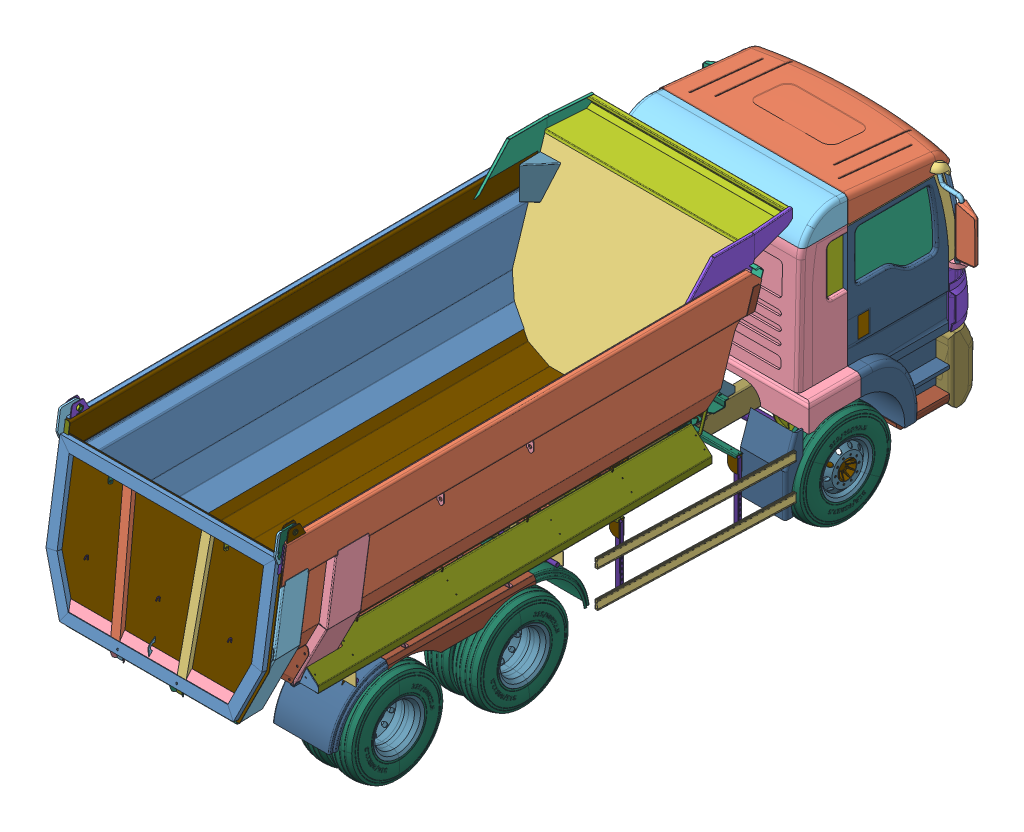
SolidWorks assembly MAN5, configuration Default. Lengths in mm. (continued)
Components (placement in the parent): (continued)
- MAN5.IGS-1: MAN5.IGS [Default] at origin size (3197.79 4674.46 9356.54) (continued)
  - M5 - erp33360_kapak üst sallama 20mm.IGS-1: M5 - erp33360_kapak üst sallama 20mm.IGS [Default] at (1250.8381 2990.2578 7990.13) x (0 0.005539 -0.999985) z (1 0 0) size (234.68 267.08 20.01)
  - M5 - erp33360_ÖZBEK SALLAMA MÝL.IGS-1: M5 - erp33360_ÖZBEK SALLAMA MÝL.IGS [Default] at (1196.3523 3240.9663 7706.3093) x (-1 0 0) z (0 0.043618 -0.999048) size (108.47 50 50)
  - M5 - erp33360_BURÇ1.IGS-1: M5 - erp33360_BURÇ1.IGS [Default] at (1169.8381 3240.9663 7706.3093) x (0 0.043618 -0.999048) z (1 0 0) size (57.01 57.11 25.54)
  - M5 - erp33360_sallama ayak.IGS-1: M5 - erp33360_sallama ayak.IGS [Default] at (1268.8381 3095.3253 7892.1663) x (0 0.005539 -0.999985) z (1 0 0) size (210.07 125.51 8.51)
  - M5 - erp33360_sallama ayak.IGS-2: M5 - erp33360_sallama ayak.IGS [Default] at (1205.8381 3095.3253 7892.1663) x (0 0.005539 -0.999985) z (1 0 0) size (210.07 125.51 8.51)
  - M5 - erp33360_BURÇ2.IGS-1: M5 - erp33360_BURÇ2.IGS [Default] at (1215.8381 3240.9663 7706.3093) x (0 0.879079 0.476677) z (1 0 0) size (57 57 45.54)
  - M5 - erp33360_BURÇ PÝMÝ.IGS-1: M5 - erp33360_BURÇ PÝMÝ.IGS [Default] at (1182.8381 3218.1971 7705.3152) x (0 -0.999048 -0.043618) z (0 0.043618 -0.999048) size (88.01 16.63 20.01)
  - M5 - erp33360_PÝM.IGS-1: M5 - erp33360_PÝM.IGS [Default] at (1182.2163 3195.6645 7744.3361) x (0 -0.043618 0.999048) z (0 -0.999048 -0.043618) size (56.72 5.64 2.41)
  - M5 - erp33360_Sallama ara parça.IGS-1: M5 - erp33360_Sallama ara parça.IGS [Default] at (1268.8381 3241.0739 7621.6777) x (-1 0 0) z (0 0.474355 -0.880334) size (55.01 80.01 5.01)
  - M5 - erp33360_kapak_Ust_Sallama_20mm_yený.IGS-1: M5 - erp33360_kapak_Ust_Sallama_20mm_yený.IGS [Default] at (1250.8381 3240.9663 7706.3093) x (0 0.006563 -0.999978) z (1 0 0) size (258.68 309.94 20.01)
  - M5 - erp33360_kapak_Ust_Sallama_20mm_yený.IGS-2: M5 - erp33360_kapak_Ust_Sallama_20mm_yený.IGS [Default] at (-1179.1619 3240.9663 7706.3093) x (0 0.006563 -0.999978) z (1 0 0) size (258.68 309.94 20.01)
  - M5 - erpAynalama33360_ÖZBEK SALLAMA MÝL.IGS-1: M5 - erpAynalama33360_ÖZBEK SALLAMA MÝL.IGS [Default] at (-1144.6762 3240.9663 7706.3093) x (1 0 0) z (0 -0.043618 0.999048) size (108.47 50 50)
  - M5 - erpAynalama33360_BURÇ1.IGS-1: M5 - erpAynalama33360_BURÇ1.IGS [Default] at (-1118.1619 3240.9663 7706.3093) x (0 0.043618 -0.999048) z (1 0 0) size (57.01 57.11 25.01)
  - M5 - erpAynalama33360_sallama ayak.IGS-1: M5 - erpAynalama33360_sallama ayak.IGS [Default] at (-1217.1619 3095.3253 7892.1663) x (0 0.005539 -0.999985) z (1 0 0) size (210.07 125.01 8.01)
  - M5 - erpAynalama33360_sallama ayak.IGS-2: M5 - erpAynalama33360_sallama ayak.IGS [Default] at (-1154.1619 3095.3253 7892.1663) x (0 0.005539 -0.999985) z (1 0 0) size (210.07 125.01 8.01)
  - M5 - erpAynalama33360_BURÇ2.IGS-1: M5 - erpAynalama33360_BURÇ2.IGS [Default] at (-1164.1619 3240.9663 7706.3093) x (0 0.879079 0.476677) z (1 0 0) size (57 57 45.54)
  - M5 - erpAynalama33360_BURÇ PÝMÝ.IGS-1: M5 - erpAynalama33360_BURÇ PÝMÝ.IGS [Default] at (-1131.1619 3218.1971 7705.3152) x (0 -0.999048 -0.043618) z (0 -0.043618 0.999048) size (88.01 16.63 20.01)
  - M5 - erpAynalama33360_PÝM.IGS-1: M5 - erpAynalama33360_PÝM.IGS [Default] at (-1130.5402 3195.6645 7744.3361) x (0 -0.043618 0.999048) z (0 0.999048 0.043618) size (56.72 5.64 2.41)
  - M5 - erpAynalama33360_Sallama ara parça.IGS-1: M5 - erpAynalama33360_Sallama ara parça.IGS [Default] at (-1217.1619 3241.0739 7621.6777) x (1 0 0) z (0 -0.474355 0.880334) size (55.01 80.01 5.01)
  - M5 - erp33360_kapak kilitleme dili.IGS-1: M5 - erp33360_kapak kilitleme dili.IGS [Default] at (-520.9865 1303.6235 8070.908) x (1 0 0) z (0 -0.050827 0.998707) size (166.16 71.61 59.75)
  - M5 - erp33360_dil iç takviye.IGS-1: M5 - erp33360_dil iç takviye.IGS [Default] at (-468.4024 1337.6943 8080.6523) x (1 0 0) z (0 -0.050827 0.998707) size (76.08 56.18 8.01)
  - M5 - erpAynalama33360_kapak kilitleme dili.IGS-1: M5 - erpAynalama33360_kapak kilitleme dili.IGS [Default] at (572.6626 1303.6235 8070.908) x (-1 0 0) z (0 0.050827 -0.998707) size (166.16 71.61 64.28)
  - M5 - erpAynalama33360_dil iç takviye.IGS-1: M5 - erpAynalama33360_dil iç takviye.IGS [Default] at (520.0785 1337.6943 8080.6523) x (-1 0 0) z (0 0.050827 -0.998707) size (76.08 56.18 8.01)
  - M5 - erp33360_kanca.IGS-1: M5 - erp33360_kanca.IGS [Default] at (-1007.12 1894.6124 3041.2431) x (-0.707107 -0.707096 -0.003916) z (0 0.005539 -0.999985) size (48.6 48.28 20.01)
  - M5 - erp33360_kanca.IGS-2: M5 - erp33360_kanca.IGS [Default] at (-1007.12 1889.3508 3991.2285) x (-0.707107 -0.707096 -0.003916) z (0 0.005539 -0.999985) size (48.6 48.28 20.01)
  - M5 - erp33360_kanca.IGS-3: M5 - erp33360_kanca.IGS [Default] at (-1007.12 1884.0892 4941.214) x (-0.707107 -0.707096 -0.003916) z (0 0.005539 -0.999985) size (48.6 48.28 20.01)
  - M5 - erp33360_kanca.IGS-4: M5 - erp33360_kanca.IGS [Default] at (-1007.12 1878.8276 5891.1994) x (-0.707107 -0.707096 -0.003916) z (0 0.005539 -0.999985) size (48.6 48.28 20.01)
  - M5 - erp33360_kanca.IGS-5: M5 - erp33360_kanca.IGS [Default] at (-1007.12 1873.566 6841.1848) x (-0.707107 -0.707096 -0.003916) z (0 0.005539 -0.999985) size (48.6 48.28 20.01)
  - M5 - erp33360_kanca.IGS-6: M5 - erp33360_kanca.IGS [Default] at (-1007.12 1869.1352 7641.1725) x (-0.707107 -0.707096 -0.003916) z (0 0.005539 -0.999985) size (48.6 48.28 20.01)
  - M5 - erp33360_kanca.IGS-7: M5 - erp33360_kanca.IGS [Default] at (-995.483 2108.1822 2887.3964) x (0 -0.303745 -0.952753) z (0.927289 0.35666 -0.113706) size (48.6 48.28 20.01)
  - M5 - erp33360_kanca.IGS-8: M5 - erp33360_kanca.IGS [Default] at (-962.1619 3328.5865 2328.3233) x (0 -0.999985 -0.005539) z (1 0 0) size (48.6 48.28 20.01)
  - M5 - erp33360_kanca.IGS-9: M5 - erp33360_kanca.IGS [Default] at (-312.1619 3328.5865 2328.3233) x (0 -0.999985 -0.005539) z (1 0 0) size (48.6 48.28 20.01)
  - M5 - erp33360_kanca.IGS-10: M5 - erp33360_kanca.IGS [Default] at (-774.1619 2086.9433 7981.607) x (0 0.150962 0.98854) z (-1 0 0) size (48.6 48.28 20.01)
  - M5 - erp33360_kanca.IGS-11: M5 - erp33360_kanca.IGS [Default] at (25.8381 2086.9433 7981.607) x (0 0.150962 0.98854) z (-1 0 0) size (48.6 48.28 20.01)
  - M5 - erp33360_kanca.IGS-12: M5 - erp33360_kanca.IGS [Default] at (825.8381 2086.9433 7981.607) x (0 0.150962 0.98854) z (-1 0 0) size (48.6 48.28 20.01)
  - M5 - erpAynalama33360_kanca.IGS-1: M5 - erpAynalama33360_kanca.IGS [Default] at (1047.1591 2108.1822 2887.3964) x (0 -0.303745 -0.952753) z (0.927289 -0.35666 0.113706) size (48.6 48.28 20.01)
  - M5 - erpAynalama33360_kanca.IGS-2: M5 - erpAynalama33360_kanca.IGS [Default] at (1058.7961 1894.6124 3041.2431) x (0.707107 -0.707096 -0.003916) z (0 -0.005539 0.999985) size (48.6 48.28 20.01)
  - M5 - erpAynalama33360_kanca.IGS-3: M5 - erpAynalama33360_kanca.IGS [Default] at (1058.7961 1889.3508 3991.2285) x (0.707107 -0.707096 -0.003916) z (0 -0.005539 0.999985) size (48.6 48.28 20.01)
  - M5 - erpAynalama33360_kanca.IGS-4: M5 - erpAynalama33360_kanca.IGS [Default] at (1058.7961 1884.0892 4941.214) x (0.707107 -0.707096 -0.003916) z (0 -0.005539 0.999985) size (48.6 48.28 20.01)
  - M5 - erpAynalama33360_kanca.IGS-5: M5 - erpAynalama33360_kanca.IGS [Default] at (1058.7961 1878.8276 5891.1994) x (0.707107 -0.707096 -0.003916) z (0 -0.005539 0.999985) size (48.6 48.28 20.01)
  - M5 - erpAynalama33360_kanca.IGS-6: M5 - erpAynalama33360_kanca.IGS [Default] at (1058.7961 1873.566 6841.1848) x (0.707107 -0.707096 -0.003916) z (0 -0.005539 0.999985) size (48.6 48.28 20.01)
  - M5 - erpAynalama33360_kanca.IGS-7: M5 - erpAynalama33360_kanca.IGS [Default] at (1058.7961 1869.1352 7641.1725) x (0.707107 -0.707096 -0.003916) z (0 -0.005539 0.999985) size (48.6 48.28 20.01)
  - M5 - erpAynalama33360_kanca.IGS-8: M5 - erpAynalama33360_kanca.IGS [Default] at (1013.8381 3328.5865 2328.3233) x (0 -0.999985 -0.005539) z (1 0 0) size (48.6 48.28 20.01)
  - M5 - erpAynalama33360_kanca.IGS-9: M5 - erpAynalama33360_kanca.IGS [Default] at (363.8381 3328.5865 2328.3233) x (0 -0.999985 -0.005539) z (1 0 0) size (48.6 48.28 20.01)
  - M5 - erp3360_kulak iç takviye.IGS-1: M5 - erp3360_kulak iç takviye.IGS [Default] at (-968.4538 1432.4795 7379.0946) x (1 0 0) z (0 -0.005539 0.999985) size (545.81 169.76 8.01)
  - M5 - erp3360_kulak iç takviye.IGS-2: M5 - erp3360_kulak iç takviye.IGS [Default] at (-968.4538 1433.6426 7169.0978) x (1 0 0) z (0 -0.005539 0.999985) size (545.81 169.76 8.01)
  - M5 - erpAynalama3360_kulak iç takviye.IGS-1: M5 - erpAynalama3360_kulak iç takviye.IGS [Default] at (1020.1299 1432.4795 7379.0946) x (-1 0 0) z (0 0.005539 -0.999985) size (545.81 169.76 8.01)
  - M5 - erpAynalama3360_kulak iç takviye.IGS-2: M5 - erpAynalama3360_kulak iç takviye.IGS [Default] at (1020.1299 1433.6426 7169.0978) x (-1 0 0) z (0 0.005539 -0.999985) size (545.81 169.76 8.01)
  - M5 - erp33360_Kulak iç L takviye.IGS-1: M5 - erp33360_Kulak iç L takviye.IGS [Default] at (685.8381 1536.3346 7100.1114) x (0 0.168191 0.985754) z (-1 0 0) size (40.01 60.01 250.01)
  - M5 - erpAynalama33360_Kulak iç L takviye.IGS-1: M5 - erpAynalama33360_Kulak iç L takviye.IGS [Default] at (685.8381 1534.4342 7443.2144) x (0 0.1791 -0.983831) z (1 0 0) size (40.01 60.01 250.01)
  - M5 - erpAynalama33360_Kulak iç L takviye.IGS-2: M5 - erpAynalama33360_Kulak iç L takviye.IGS [Default] at (-634.162 1536.3346 7100.1114) x (0 0.168191 0.985754) z (-1 0 0) size (40.01 60.01 250.01)
  - M5 - erpAynalamaAynalama33360_Kulak iç L takviye.IGS-1: M5 - erpAynalamaAynalama33360_Kulak iç L takviye.IGS [Default] at (-634.162 1534.4342 7443.2144) x (0 0.1791 -0.983831) z (1 0 0) size (40.01 60.01 250.01)
  - M5 - erp33360_takviye 3.IGS-1: M5 - erp33360_takviye 3.IGS [Default] at (496.575 1458.2519 7075.2326) x (-1 0 0) z (0 0.005539 -0.999985) size (707.09 63.73 70.86)
  - M5 - erpAynalama33360_takviye 3.IGS-1: M5 - erpAynalama33360_takviye 3.IGS [Default] at (496.575 1456.0808 7467.2266) x (-1 0 0) z (0 0.005539 -0.999985) size (707.09 63.73 70.86)
  - M5 - erp33360_takviye 2.IGS-1: M5 - erp33360_takviye 2.IGS [Default] at (-1807.7153 1265.8802 7061.7989) x (0.99991 -0.000074 0.013388) z (-0.013388 -0.000196 0.99991) size (761.79 408.47 64.91)
  - M5 - erp33360_takviye 2.IGS-2: M5 - erp33360_takviye 2.IGS [Default] at (-1807.7153 1263.6925 7456.7928) x (0.99991 -0.000074 0.013388) z (-0.013388 -0.000196 0.99991) size (761.79 408.47 64.91)
  - M5 - erp33360_takviye 1.IGS-1: M5 - erp33360_takviye 1.IGS [Default] at (-1188.2366 1554.8437 7093.9387) x (1 0 0) z (0 0.194032 0.980995) size (498.01 334.11 6.01)
  - M5 - erp33360_takviye 1.IGS-2: M5 - erp33360_takviye 1.IGS [Default] at (-1189.0116 1551.4786 7467.5378) x (1 0 0) z (0 0.177892 0.98405) size (498.01 334.11 6.01)
  - M5 - erp33360_takviye 1.IGS-3: M5 - erp33360_takviye 1.IGS [Default] at (-1190.4757 1549.1198 8040.8256) x (1 0 0) z (0 0.15315 0.988203) size (498.01 334.11 6.01)
  - M5 - erpAynalama33360_takviye 1.IGS-1: M5 - erpAynalama33360_takviye 1.IGS [Default] at (1240.6877 1551.4786 7467.5378) x (-1 0 0) z (0 -0.177892 -0.98405) size (498.01 334.11 6.01)
  - M5 - erpAynalama33360_takviye 1.IGS-2: M5 - erpAynalama33360_takviye 1.IGS [Default] at (1239.9127 1554.8437 7093.9387) x (-1 0 0) z (0 -0.194032 -0.980995) size (498.01 334.11 6.01)
  - M5 - erpAynalama33360_takviye 1.IGS-3: M5 - erpAynalama33360_takviye 1.IGS [Default] at (1242.1518 1549.1198 8040.8256) x (-1 0 0) z (0 -0.15315 -0.988203) size (498.01 334.11 6.01)
  - M5 - erpAynalama33360_takviye 2.IGS-1: M5 - erpAynalama33360_takviye 2.IGS [Default] at (1859.3914 1263.6925 7456.7928) x (-0.99991 -0.000074 0.013388) z (-0.013388 0.000196 -0.99991) size (761.85 408.18 64.62)
  - M5 - erpAynalama33360_takviye 2.IGS-2: M5 - erpAynalama33360_takviye 2.IGS [Default] at (1859.3914 1265.8802 7061.7989) x (-0.99991 -0.000074 0.013388) z (-0.013388 0.000196 -0.99991) size (761.85 408.18 64.62)
  - M5 - erp33360_kros köþe takviye.IGS-1: M5 - erp33360_kros köþe takviye.IGS [Default] at (76001.9762 -57131.283 18206.8496) x (0.999704 -0.016093 0.018269) z (-0.015329 0.166915 0.985852) size (126.6 251.73 5.21)
  - M5 - erp33360_kros köþe takviye.IGS-2: M5 - erp33360_kros köþe takviye.IGS [Default] at (76001.9762 -57133.4596 18599.8436) x (0.999704 -0.016093 0.018269) z (-0.015329 0.166915 0.985852) size (126.6 251.73 5.21)
  - M5 - erp33360_kros köþe takviye.IGS-3: M5 - erp33360_kros köþe takviye.IGS [Default] at (76001.9762 -57135.8135 19024.8371) x (0.999704 -0.016093 0.018269) z (-0.015329 0.166915 0.985852) size (126.6 251.73 5.21)
  - M5 - erp33360_kros köþe takviye.IGS-4: M5 - erp33360_kros köþe takviye.IGS [Default] at (76001.9762 -57136.683 19181.8347) x (0.999704 -0.016093 0.018269) z (-0.015329 0.166915 0.985852) size (126.6 251.73 5.21)
  - M5 - erp33360_kros iç takviyeler.IGS-1: M5 - erp33360_kros iç takviyeler.IGS [Default] at (-1141.7209 2140.6998 6983.7472) x (-0.115396 0.970111 -0.213467) z (-0.007467 0.21405 0.976794) size (80.01 50.01 5.01)
  - M5 - erp33360_kros iç takviyeler.IGS-2: M5 - erp33360_kros iç takviyeler.IGS [Default] at (-1141.7209 2137.9288 7350.7367) x (-0.115396 0.970111 -0.213467) z (-0.007467 0.21405 0.976794) size (80.01 50.01 5.01)
  - M5 - erp33360_kros iç takviyeler.IGS-3: M5 - erp33360_kros iç takviyeler.IGS [Default] at (-1141.7209 2134.5161 7802.7238) x (-0.115396 0.970111 -0.213467) z (-0.007467 0.21405 0.976794) size (80.01 50.01 5.01)
  - M5 - erp33360_kros iç takviyeler.IGS-4: M5 - erp33360_kros iç takviyeler.IGS [Default] at (-1141.7209 2130.1615 7935.6525) x (-0.115396 0.970111 -0.213467) z (-0.007467 0.21405 0.976794) size (80.01 50.01 5.01)
  - M5 - erpAynalama33360_kros köþe takviye.IGS-1: M5 - erpAynalama33360_kros köþe takviye.IGS [Default] at (-75950.3001 -57135.8135 19024.8371) x (-0.999704 -0.016093 0.018269) z (-0.015329 -0.166915 -0.985852) size (126.46 251.73 5.03)
  - M5 - erpAynalama33360_kros köþe takviye.IGS-2: M5 - erpAynalama33360_kros köþe takviye.IGS [Default] at (-75950.3001 -57136.683 19181.8347) x (-0.999704 -0.016093 0.018269) z (-0.015329 -0.166915 -0.985852) size (126.46 251.73 5.03)
  - M5 - erpAynalama33360_kros iç takviyeler.IGS-1: M5 - erpAynalama33360_kros iç takviyeler.IGS [Default] at (1193.397 2130.1615 7935.6525) x (0.115396 0.970111 -0.213467) z (-0.007467 -0.21405 -0.976794) size (80.01 50.01 5.01)
  - M5 - erpAynalama33360_kros iç takviyeler.IGS-2: M5 - erpAynalama33360_kros iç takviyeler.IGS [Default] at (1193.397 2134.5161 7802.7238) x (0.115396 0.970111 -0.213467) z (-0.007467 -0.21405 -0.976794) size (80.01 50.01 5.01)
  - M5 - erpAynalama33360_kros iç takviyeler.IGS-3: M5 - erpAynalama33360_kros iç takviyeler.IGS [Default] at (1193.397 2137.9288 7350.7367) x (0.115396 0.970111 -0.213467) z (-0.007467 -0.21405 -0.976794) size (80.01 50.01 5.01)
  - M5 - erpAynalama33360_kros iç takviyeler.IGS-4: M5 - erpAynalama33360_kros iç takviyeler.IGS [Default] at (1193.397 2140.6998 6983.7472) x (0.115396 0.970111 -0.213467) z (-0.007467 -0.21405 -0.976794) size (80.01 50.01 5.01)
  - M5 - erp33360_merdiven kenar.IGS-1: M5 - erp33360_merdiven kenar.IGS [Default] at (-1236.3747 1422.6306 3114.9753) x (0 -0.005539 0.999985) z (-1 0 0) size (299.61 1419.81 27.01)
  - M5 - erp33360_merdiven kenar.IGS-2: M5 - erp33360_merdiven kenar.IGS [Default] at (1008.6439 1695.0904 2922.4949) x (-0.999988 0.004679 -0.001484) z (0 -0.302356 -0.953195) size (299.61 1419.81 27.01)
  - M5 - erp33360_basamak.IGS-1: M5 - erp33360_basamak.IGS [Default] at (-1238.8747 1686.7214 3373.435) x (0.383813 0.923397 0.005114) z (0 0.005539 -0.999985) size (32.01 32.01 250.01)
  - M5 - erp33360_basamak.IGS-2: M5 - erp33360_basamak.IGS [Default] at (-1238.8747 1986.7168 3375.0965) x (0.383813 0.923397 0.005114) z (0 0.005539 -0.999985) size (32.01 32.01 250.01)
  - M5 - erp33360_basamak.IGS-3: M5 - erp33360_basamak.IGS [Default] at (-1238.8747 2286.7122 3376.7581) x (0.383813 0.923397 0.005114) z (0 0.005539 -0.999985) size (32.01 32.01 250.01)
  - M5 - erp33360_basamak.IGS-4: M5 - erp33360_basamak.IGS [Default] at (-1238.8747 2586.7076 3378.4196) x (0.383813 0.923397 0.005114) z (0 0.005539 -0.999985) size (32.01 32.01 250.01)
  - M5 - erp33360_basamak.IGS-5: M5 - erp33360_basamak.IGS [Default] at (752.9573 1948.6246 2839.4504) x (0.004533 0.996228 0.086653) z (0.999988 -0.004679 0.001484) size (32.01 32.01 250.01)
  - M5 - erp33360_basamak.IGS-6: M5 - erp33360_basamak.IGS [Default] at (754.43 2234.5796 2748.7445) x (0.004533 0.996228 0.086653) z (0.999988 -0.004679 0.001484) size (32.01 32.01 250.01)
  - M5 - erp33360_basamak.IGS-7: M5 - erp33360_basamak.IGS [Default] at (755.9026 2520.5347 2658.0387) x (0.004533 0.996228 0.086653) z (0.999988 -0.004679 0.001484) size (32.01 32.01 250.01)
  - M5 - erp33360_basamak.IGS-8: M5 - erp33360_basamak.IGS [Default] at (757.3752 2806.4897 2567.3329) x (0.004533 0.996228 0.086653) z (0.999988 -0.004679 0.001484) size (32.01 32.01 250.01)
  - M5 - erp33360_merdiven kulaðý.IGS-1: M5 - erp33360_merdiven kulaðý.IGS [Default] at (-1280.2341 2665.318 3121.8511) x (1 0 0) z (0 -0.005539 0.999985) size (37.43 58.66 6.01)
  - M5 - erp33360_merdiven kulaðý.IGS-2: M5 - erp33360_merdiven kulaðý.IGS [Default] at (-1280.2341 2663.8115 3393.8469) x (1 0 0) z (0 -0.005539 0.999985) size (37.43 58.66 6.01)
  - M5 - erp33360_merdiven kulaðý.IGS-3: M5 - erp33360_merdiven kulaðý.IGS [Default] at (-1232.7968 2889.017 3129.0901) x (-0.615661 -0.787999 -0.004364) z (0 -0.005539 0.999985) size (37.43 58.66 6.01)
  - M5 - erp33360_merdiven kulaðý.IGS-4: M5 - erp33360_merdiven kulaðý.IGS [Default] at (-1232.7968 2887.577 3389.0862) x (-0.615661 -0.787999 -0.004364) z (0 -0.005539 0.999985) size (37.43 58.66 6.01)
  - M5 - erp33360_merdiven kulaðý.IGS-5: M5 - erp33360_merdiven kulaðý.IGS [Default] at (1014.751 2866.3565 2504.9526) x (0 0.302356 0.953195) z (-0.999988 0.004679 -0.001484) size (37.43 58.66 6.01)
  - M5 - erp33360_merdiven kulaðý.IGS-6: M5 - erp33360_merdiven kulaðý.IGS [Default] at (742.7542 2867.6291 2504.5489) x (0 0.302356 0.953195) z (-0.999988 0.004679 -0.001484) size (37.43 58.66 6.01)
  - M5 - erp33360_Emniyet kolu kasa parçasý1.IGS-1: M5 - erp33360_Emniyet kolu kasa parçasý1.IGS [Default] at (-480.4872 1623.7217 5522.1253) x (1 0 0) z (0 0.005539 -0.999985) size (70.01 55.01 50.01)
  - M5 - erp33360_Emniyet kolu kasa parçasý2.IGS-1: M5 - erp33360_Emniyet kolu kasa parçasý2.IGS [Default] at (-480.4872 1623.9986 5472.1261) x (1 0 0) z (0 0.005539 -0.999985) size (62.01 51.01 4.01)
  - M5 - erp33360_Emniyet kolu kasa parçasý2.IGS-2: M5 - erp33360_Emniyet kolu kasa parçasý2.IGS [Default] at (-480.4872 1623.7439 5518.1253) x (1 0 0) z (0 0.005539 -0.999985) size (62.01 51.01 4.01)
  - M5 - erp33360_mapa.IGS-1: M5 - erp33360_mapa.IGS [Default] at (-955.2293 2577.4542 5026.871) x (-1 0 0) z (0 0.005539 -0.999985) size (73.94 131.22 10.01)
  - M5 - erp33360_mapa.IGS-2: M5 - erp33360_mapa.IGS [Default] at (-955.2293 2571.9157 6026.8557) x (-1 0 0) z (0 0.005539 -0.999985) size (73.94 131.22 10.01)
  - M5 - erpAynalama33360_mapa.IGS-1: M5 - erpAynalama33360_mapa.IGS [Default] at (1006.9054 2577.4542 5026.871) x (1 0 0) z (0 -0.005539 0.999985) size (73.94 131.22 10.01)
  - M5 - erpAynalama33360_mapa.IGS-2: M5 - erpAynalama33360_mapa.IGS [Default] at (1006.9054 2571.9157 6026.8557) x (1 0 0) z (0 -0.005539 0.999985) size (73.94 131.22 10.01)
  - AynalamaM5 - erp33360_ÖZBEKÝSTAN küçük yan kros.IGS-1: AynalamaM5 - erp33360_ÖZBEKÝSTAN küçük yan kros.IGS [Default] at (1293.8804 1026.8349 7834.3506) x (0 0.150962 0.98854) z (0 -0.98854 0.150962) size (842.09 416.57 1466.67)
  - AynalamaM5 - erp33360_ÖZBEKÝSTAN öngöðüs kuþak krosu.IGS-1: AynalamaM5 - erp33360_ÖZBEKÝSTAN öngöðüs kuþak krosu.IGS [Default] at (1269.7184 -352742.0932 105385.5445) x (0 0.953195 -0.302356) z (1 0 0) size (367.53 86.57 1017.75)
  - Kopya [MA]  Part_PISTON GHS 175-5-5550 C^M5 - Model_004_merkez.IGS-1: Kopya [MA]  Part_PISTON GHS 175-5-5550 C^M5 - Model_004_merkez.IGS [Default] at (25.8332 1735.5904 2819.8799) x (0 0.291338 0.95662) z (-1 0 0) size (262.9 1690.31 360.01)
